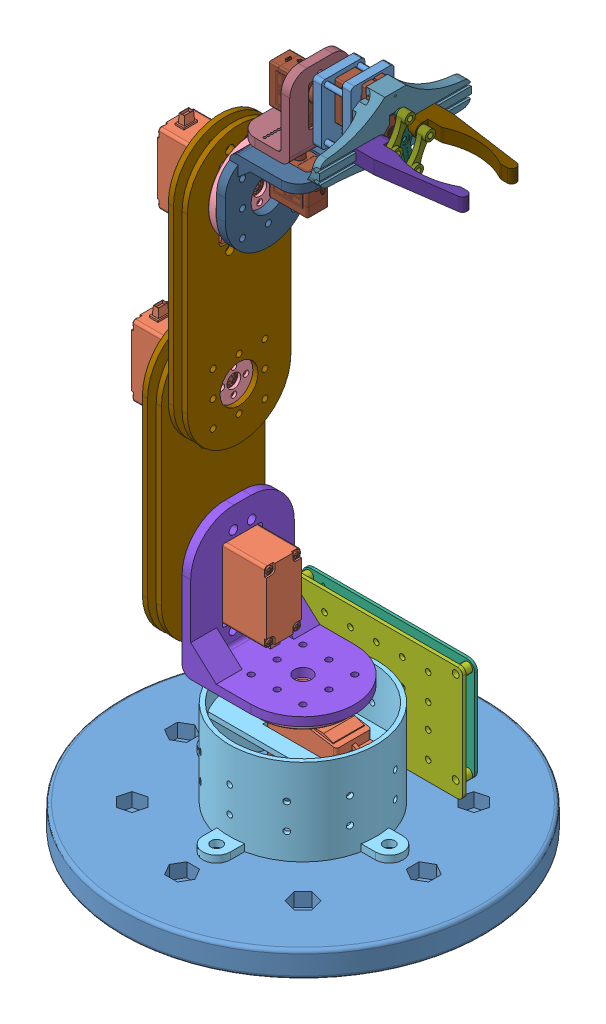
SolidWorks assembly main, configuration Default. Lengths in mm.
Overall size (214.3 404.54 210).
55 component instances, 20 part files, 29 mates.
Components (placement in the parent):
- robot_base-1: robot_base [Default] at origin size (210 15 210)
- Base^main-1: Base^main [Default] at (0.0003 7.5 0) size (116 70 116) (virtual, flexible)
  - 1501MG_adapter-1: 1501MG_adapter [Default] at (29.5503 10 -10.25) size (61.65 49 50) (flexible)
    - 1501MG_assem-1: 1501MG_assem [Default] x (-1 0 0) z (0 0 -1) size (55 46 20.5) (flexible)
      - ServoHD1501MG-1: ServoHD1501MG [Default] x (1 0 0) z (0 1 0) size (55 21 47.7)
      - Servo Output Shaft-1: Servo Output Shaft [Default] at (29.55 36.5 -10.25) size (6 9 6) (hidden)
      - ServoHD1501MG_horn-1: ServoHD1501MG_horn [Default] at (29.55 46 -10.25) x (1 0 0) z (0 -1 0) size (20 20 4.5)
    - base-1: base [Default] at (-29.55 46.5 10.25) x (1 0 0) z (0 0 -1) size (50 5 50)
  - base_round-1: base_round [Default] at origin size (116 50 116)
  - OBJ_PCB_Manip-1: OBJ_PCB_Manip [Default] at (-50 70 -51.1) size (100 60 1.6)
  - pcbHOlder-1: pcbHOlder [Default] at (0 37 -44.5) size (100 66 7)
- link0^main-1: link0^main [Default] at (-17.4995 66.5 0) x (0 -1 0) z (0 0 -1) size (78.35 90 63.4) (virtual)
  - 1501MG_adapter-1: 1501MG_adapter [Default] at (-57.9 -6.5 10.25) x (-1 0 0) z (0 0 -1) size (67 49 60.7) (flexible)
    - 1501MG_assem-1: 1501MG_assem [Default] x (-1 0 0) z (0 0 -1) size (55 46 27.64) (flexible)
      - ServoHD1501MG-1: ServoHD1501MG [Default] x (1 0 0) z (0 1 0) size (55 21 47.7)
      - Servo Output Shaft-1: Servo Output Shaft [Default] at (29.55 36.5 -10.25) x (0.320733 0 0.94717) z (-0.94717 0 0.320733) size (6 9 6) (hidden)
      - ServoHD1501MG_horn-1: ServoHD1501MG_horn [Default] at (29.55 46 -10.25) x (0.320733 0 0.94717) z (0 -1 0) size (20 20 4.5)
    - base-1: base [Default] at (-29.55 46.5 10.25) x (0.320733 0 0.94717) z (0.94717 0 -0.320733) size (50 5 50)
  - link_90-1: link_90 [Default] x (-1 0 0) z (0 0 -1) size (75 70 60)
- Link1^main-1: Link1^main [Default] at (-88.9995 169.3 -10.25) x (0 1 0) z (0 0 -1) size (169.12 49 70.25) (virtual, flexible)
  - link-1: link [Default] at (-24.45 34 -10.25) x (0 1 0) z (0 0 -1) size (3 160 60)
  - 1501MG_adapter-1: 1501MG_adapter [Default] x (-1 0 0) z (0 0 -1) size (67 49 60.7) (flexible)
    - 1501MG_assem-1: 1501MG_assem [Default] x (-1 0 0) z (0 0 -1) size (55 46 27.64) (flexible)
      - ServoHD1501MG-1: ServoHD1501MG [Default] x (1 0 0) z (0 1 0) size (55 21 47.7)
      - Servo Output Shaft-1: Servo Output Shaft [Default] at (29.55 36.5 -10.25) x (0 0 -1) z (1 0 0) size (6 9 6) (hidden)
      - ServoHD1501MG_horn-1: ServoHD1501MG_horn [Default] at (29.55 46 -10.25) x (0 0 -1) z (0 -1 0) size (20 20 4.5)
    - base-1: base [Default] at (-29.55 46.5 10.25) x (0 0 -1) z (-1 0 0) size (50 5 50)
  - link-2: link [Default] at (-24.45 26 -10.25) x (0 1 0) z (0 0 -1) size (3 160 60)
- Link2^main-1: Link2^main [Default] at (-73.9995 273.3 -10.25) x (0 -1 0) z (0 0 -1) size (163.02 49 60) (virtual, flexible)
  - link-1: link [Default] at (24.45 -34 -10.25) x (0 -1 0) z (0 0 -1) size (3 160 60)
  - link-2: link [Default] at (24.45 -26 -10.25) x (0 -1 0) z (0 0 -1) size (3 160 60)
  - 1501MG_adapter-1: 1501MG_adapter [Default] x (1 0 0) z (0 0 -1) size (67 49 60.7) (flexible)
    - 1501MG_assem-1: 1501MG_assem [Default] x (-1 0 0) z (0 0 -1) size (55 46 27.64) (flexible)
      - ServoHD1501MG-1: ServoHD1501MG [Default] x (1 0 0) z (0 1 0) size (55 21 47.7)
      - Servo Output Shaft-1: Servo Output Shaft [Default] at (29.55 36.5 -10.25) size (6 9 6) (hidden)
      - ServoHD1501MG_horn-1: ServoHD1501MG_horn [Default] at (29.55 46 -10.25) x (1 0 0) z (0 -1 0) size (20 20 4.5)
    - base-1: base [Default] at (-29.55 46.5 10.25) x (1 0 0) z (0 0 -1) size (50 5 50)
- link3^main-1: link3^main [Default] at (241.0039 142.2283 119.15) x (0 0 1) z (-0.674726 -0.738069 0) size (50 66.63 70.3) (virtual, flexible)
  - link_90_small-1: link_90_small [Default] at (-119.15 311.7889 53.1797) x (0 -0.738069 -0.674726) z (1 0 0) size (40 55 50)
  - SG90 - Micro Servo 9g - Tower Pro-1: SG90 - Micro Servo 9g - Tower Pro [Default] at (-146.9332 292.0328 51.3341) x (0 -0.738069 -0.674726) z (1 0 0) size (32.6 32.03 12.4)
  - SG90 - Micro Servo 9g - Tower Pro.3-1: SG90 - Micro Servo 9g - Tower Pro.3 [Peça] at (-119.15 316.4926 22.3204) x (-1 0 0) z (0 -0.738069 -0.674726) size (32.1 3.8 6.9)
- link4^main-1: link4^main [Default] at (264.2022 318.2362 -212.0717) x (0.275398 -0.96133 0) z (-0.648634 -0.185818 -0.738069) size (51.52 54.05 53.65) (virtual, flexible)
  - link_90_small_short-1: link_90_small_short [Default] at (-95.1167 331.695 15.8948) x (-0.96133 -0.203263 -0.185818) z (0 -0.674726 0.738069) size (45 30 35)
  - SG90 - Micro Servo 9g - Tower Pro-1: SG90 - Micro Servo 9g - Tower Pro [Default] at (-128.8611 315.0024 38.2779) x (0.96133 0.203263 0.185818) z (0 0.674726 -0.738069) size (32.6 32.03 12.4)
  - SG90 - Micro Servo 9g - Tower Pro.3-1: SG90 - Micro Servo 9g - Tower Pro.3 [Peça] at (-116.9543 307.1544 -6.5397) x (-0.96133 -0.203263 -0.185818) z (0 -0.674726 0.738069) size (32.1 3.8 6.9)
- Gripper^main-1: Gripper^main [Default] at (18.3005 369.45 0) x (1 0 0) z (0 -1 0) size (91 87.8 40) (virtual, flexible)
  - Linear Gripper-1: Linear Gripper [Default] at (11.6 15.2 -5.1547) x (1 0 0) z (0 -1 0) size (89.03 54.99 87.8) (flexible)
    - Linear Base-1: Linear Base [Default] at origin size (11.05 33.39 87.8)
    - SG90 - Micro Servo 9g - Tower Pro-2: SG90 - Micro Servo 9g - Tower Pro [Default] at (-11.5678 6.678 -12.5832) x (0 -1 0) z (0 0 1) size (32.6 32.03 12.4)
    - Horn-1: Horn [По умолчанию] at (29.55 5.1547 15.2) x (0 -0.986664 -0.162773) z (-1 0 0) size (32 7.5 5)
    - gripper_linear_link-1: gripper_linear_link [Default] at (31.05 12.333 21.0801) x (0 0.896643 -0.442754) z (1 0 0) size (21.9 6 5)
    - gripper_linear_link-2: gripper_linear_link [Default] at (31.05 -2.0236 9.3199) x (0 0.896643 -0.442754) z (1 0 0) size (21.9 6 5)
    - gripper_grip-2: gripper_grip [Default] at (26.2 4.0581 -2.7) x (0 0 1) z (-1 0 0) size (17.35 8.47 59.1)
    - Mirrorgripper_grip-3: Mirrorgripper_grip [Default] at (26.2 4.0581 33.1) x (0 0 -1) z (1 0 0) size (17.35 8.47 59.1)
  - ee_link-1: ee_link [Default] at origin size (22 25 40)
Mates (geometry in assembly coordinates):
- Coincident48: coincident anti-aligned: plane of Link1^main2-1/1501MG_adapter-1/base-1 through (-39.9995 198.85 0) normal (1 0 0); plane of Link2^main2-1/link-1 through (-39.9995 248.85 0) normal (-1 0 0)
- Concentric54: concentric aligned: cylinder of Link1^main2-1/1501MG_adapter-1/base-1 through (-45.0005 198.85 -15) axis (1 0 0) radius 1.65; cylinder of Link2^main2-1/link-1 through (-40.0005 198.85 -15) axis (1 0 0) radius 1.75
- Concentric55: concentric aligned: cylinder of Link1^main2-1/1501MG_adapter-1/base-1 through (-45.0005 213.85 -15) axis (1 0 0) radius 1.65; cylinder of Link2^main2-1/link-1 through (-40.0005 213.85 -15) axis (1 0 0) radius 1.75
- Coincident51: coincident anti-aligned: plane of Link2^main2-1/1501MG_adapter-1/base-1 through (-24.9995 302.85 0) normal (1 0 0); plane of link3^main2-1/link_90_small-1 through (-24.9995 313.35 0) normal (-1 0 0)
- Concentric58: concentric aligned: cylinder of Link2^main2-1/1501MG_adapter-1/base-1 through (-30.0005 287.85 0) axis (1 0 0) radius 1.65; cylinder of link3^main2-1/link_90_small-1 through (-25.0005 287.85 0) axis (1 0 0) radius 1.75
- Concentric59: concentric aligned: cylinder of Link2^main2-1/1501MG_adapter-1/base-1 through (-30.0005 302.85 15) axis (1 0 0) radius 1.65; cylinder of link3^main2-1/link_90_small-1 through (-25.0005 302.85 15) axis (1 0 0) radius 1.75
- Concentric62: concentric anti-aligned: cylinder of link4^main2-1/link_90_small_short-1 through (-7.6495 344.3 -14.45) axis (0 -1 0) radius 0.75; cylinder of link3^main2-1/SG90 - Micro Servo 9g - Tower Pro.3-1 through (-7.6495 339.3 -14.45) axis (0 1 0) radius 0.6
- Coincident53: coincident anti-aligned: plane of link4^main2-1/link_90_small_short-1 through (-7.6495 339.3 0) normal (0 -1 0); plane of link3^main2-1/SG90 - Micro Servo 9g - Tower Pro.3-1 through (-7.6495 339.3 0) normal (0 1 0)
- Concentric63: concentric anti-aligned: cylinder of link4^main2-1/link_90_small_short-1 through (-7.6495 344.3 14.45) axis (0 -1 0) radius 0.75; cylinder of link3^main2-1/SG90 - Micro Servo 9g - Tower Pro.3-1 through (-7.6495 339.3 14.45) axis (0 1 0) radius 0.6
- Coincident64: coincident anti-aligned: plane of Base^main2-1/1501MG_adapter-1/base-1 through (0.0005 66.5 0) normal (0 1 0); plane of link0^main-1/link_90-1 through (-17.4995 66.5 0) normal (0 -1 0)
- Concentric72: concentric aligned: cylinder of Base^main2-1/1501MG_adapter-1/base-1 through (15.0005 61.499 15) axis (0 1 0) radius 1.65; cylinder of link0^main-1/link_90-1 through (15.0005 66.499 15) axis (0 1 0) radius 1.75
- Concentric73: concentric aligned: cylinder of Base^main2-1/1501MG_adapter-1/base-1 through (15.0005 61.499 0) axis (0 1 0) radius 1.65; cylinder of link0^main-1/link_90-1 through (15.0005 66.499 0) axis (0 1 0) radius 1.75
- Concentric76: concentric anti-aligned: cylinder of Gripper^main2-1/ee_link-1 through (23.3005 375.9 0) axis (-1 0 0) radius 0.75; cylinder of link4^main2-1/SG90 - Micro Servo 9g - Tower Pro.3-1 through (18.3005 375.9 0) axis (1 0 0) radius 0.6
- Coincident67: coincident anti-aligned: plane of link4^main2-1/SG90 - Micro Servo 9g - Tower Pro.3-1 through (18.3005 369.45 0) normal (1 0 0); plane of Gripper^main2-1/ee_link-1 through (18.3005 369.45 0) normal (-1 0 0)
- Concentric77: concentric anti-aligned: cylinder of link4^main2-1/SG90 - Micro Servo 9g - Tower Pro.3-1 through (18.3005 359 0) axis (1 0 0) radius 0.6; cylinder of Gripper^main2-1/ee_link-1 through (23.3005 359 0) axis (-1 0 0) radius 0.75
- Concentric78: concentric anti-aligned: cylinder of Base^main-1/base_round-1 through (-50 11.5 0) axis (0 -1 0) radius 3.25; cylinder of robot_base-1 through (-50 -7.5 0) axis (0 1 0) radius 3.5
- Concentric79: concentric anti-aligned: cylinder of Base^main-1/base_round-1 through (50.0005 11.5 0) axis (0 -1 0) radius 3.25; cylinder of robot_base-1 through (50 -7.5 0) axis (0 1 0) radius 3.5
- Coincident68: coincident anti-aligned: plane of Base^main-1/base_round-1 through (0.0003 7.5 0) normal (0 -1 0); plane of robot_base-1 through (0 7.5 0) normal (0 1 0)
- Coincident69: coincident aligned: plane of robot_base-1 through (0 0 0) normal (0 0 1)
- Coincident70: coincident aligned: plane of robot_base-1 through (0 0 0) normal (0 1 0)
- Coincident71: coincident aligned: plane of robot_base-1 through (0 0 0) normal (1 0 0)
- Concentric80: concentric anti-aligned: cylinder of link0^main2-1/1501MG_adapter-1/base-1 through (-54.9995 94.85 0) axis (-1 0 0) radius 25; cylinder of Link1^main2-1/link-2 through (-63.0005 94.85 0) axis (1 0 0) radius 11
- Coincident72: coincident anti-aligned: plane of link0^main2-1/1501MG_adapter-1/base-1 through (-54.9995 94.85 0) normal (1 0 0); plane of Link1^main2-1/link-1 through (-54.9995 144.85 0) normal (-1 0 0)
- Angle2: planar angle aligned: plane of link0^main-1/link_90-1 through (-17.4995 71.5 -30) normal (0 0 -1); plane of Base^main-1/base_round-1 through (34.0003 46.5 -21.0713) normal (0 0 -1)
- Angle1: planar angle anti-aligned: plane of link0^main-1/link_90-1 through (-17.4995 71.5 -30) normal (0 0 -1); plane of Link1^main2-1/link-2 through (-59.9995 144.85 30) normal (0 0 1)
- Angle3: planar angle anti-aligned: plane of Link2^main2-1/link-1 through (-36.9995 248.85 30) normal (0 0 1); plane of Link1^main2-1/link-1 through (-51.9995 144.85 30) normal (0 0 1)
- Angle5: planar angle anti-aligned: plane of link3^main2-1/link_90_small-1 through (-19.9995 313.35 25) normal (0 0 1); plane of Link2^main2-1/link-1 through (-36.9995 248.85 30) normal (0 0 1)
- Angle6: planar angle anti-aligned: plane of link3^main2-1/link_90_small-1 through (-24.9995 330.85 17.5) normal (0 0 1); plane of link4^main2-1/link_90_small_short-1 through (-7.6495 344.3 17.5) normal (0 0 1)
- Angle7: planar angle anti-aligned: plane of Gripper^main2-1/ee_link-1 through (23.3005 386.95 0) normal (0 1 0); plane of link4^main2-1/link_90_small_short-1 through (9.8505 384.3 17.5) normal (0 1 0)
